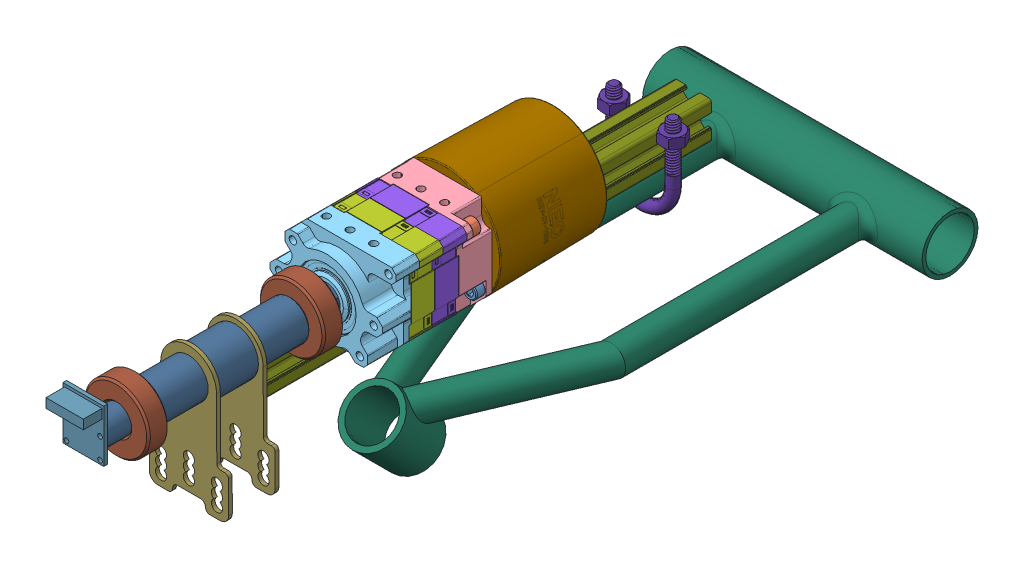
SolidWorks assembly SBW lower asm, configuration Default. Lengths in mm.
Overall size (161.8 159.3 415).
29 component instances, 20 part files, 63 mates.
Components (placement in the parent):
- MAXPlanetary 2-Stage-1: MAXPlanetary 2-Stage [Default] at origin size (89.61 89.51 122.08)
  - MAXPlanetary 2-Stage.STEP-1: MAXPlanetary 2-Stage.STEP [Default] at origin size (89.61 89.51 122.08)
    - REV-25-2109_2-Stage (No Shaft, For NEO).STEP-1: REV-25-2109_2-Stage (No Shaft, For NEO).STEP [Default] at origin size (65.15 54.03 73.34)
      - REV-25-2107_2-Stage.STEP-1: REV-25-2107_2-Stage.STEP [Default] at (0 0 6.35) x (-1 0 0) z (0 0 -1) size (65.15 54.03 73.34)
        - #10 Socket Head Cap Screws_0.500in Long.STEP-1: #10 Socket Head Cap Screws_0.500in Long.STEP [Default] at (21.1355 14.0872 12.7) x (0.923728 0.383049 0) z (0.383049 -0.923728 0) size (7.94 17.53 7.94)
        - #10 Socket Head Cap Screws_0.500in Long.STEP-2: #10 Socket Head Cap Screws_0.500in Long.STEP [Default] at (-21.1355 -14.0872 12.7) x (0.923728 0.383049 0) z (0.383049 -0.923728 0) size (7.94 17.53 7.94)
        - #10 Socket Head Cap Screws_1.500in Long.STEP-1: #10 Socket Head Cap Screws_1.500in Long.STEP [Default] at (-26.9919 21.4312 0) x (0.777574 0.628792 0) z (-0.628792 0.777574 0) size (7.94 42.93 7.94)
        - #10 Socket Head Cap Screws_1.500in Long.STEP-2: #10 Socket Head Cap Screws_1.500in Long.STEP [Default] at (26.9919 -21.4312 0) x (0.777574 0.628792 0) z (-0.628792 0.777574 0) size (7.94 42.93 7.94)
        - #10-32 Button Head Cap Screws_0.500in Long.STEP-1: #10-32 Button Head Cap Screws_0.500in Long.STEP [Default] at (0 0 -35.2425) x (0.655967 -0.754789 0) z (-0.754789 -0.655967 0) size (9.17 15.27 9.17)
      - REV-21-2106.STEP-1: REV-21-2106.STEP [Default] at origin size (61.91 50.8 19.05)
      - REV-21-2104.STEP-1: REV-21-2104.STEP [Default] at (0 0 44.45) x (0 0 1) z (-1 0 0) size (23.2 50.8 61.92)
      - REV-21-2108.STEP-1: REV-21-2108.STEP [Default] at (0 0 7.0985) x (-0.554615 -0.832107 0) z (0 0 -1) size (25.4 25.4 14.94)
    - REV-21-2101.STEP-1: REV-21-2101.STEP [Default] at (0 0 28.575) size (61.91 50.8 16.85)
    - REV-21-2102.STEP-1: REV-21-2102.STEP [Default] at (0 0 15.875) size (61.91 50.8 16.85)
    - REV-21-1650.STEP-1: REV-21-1650.STEP [Default] at (0 0 -9.525) x (0.554615 0.832107 0) z (0 0 1) size (64.41 64.76 93.26)
- shaft-1: shaft [Default] at (0 0 42.8625) x (0 0 1) z (-0.999764 0.021721 0) size (138 25 25)
- deep groove bearing 6202-1: deep groove bearing 6202 [默认] at (0 0 61.8625) size (35 35 11)
- shaft link-1: shaft link [默认] at (0 0 100.8625) x (0.999993 0.003842 0) z (0 0 1) size (42.5 73 2)
- shaft link-2: shaft link [默认] at (0 0 125.8625) x (0.999993 0.003842 0) z (0 0 1) size (42.5 73 2)
- AS5047P magnet-1: AS5047P magnet [Default] at (0 0 180.8625) x (1 0 0) z (0 1 0) size (6 2.5 6)
- deep groove bearing 6202-2: deep groove bearing 6202 [默认] at (0 0 155.8625) size (35 35 11)
- AS5047P-1: AS5047P [Default] at (0 6.4979 182.3625) size (22 28 12)
- lower AS5047P mount-1: lower AS5047P mount [Default] at (0 0 189.3625) x (0 0 -1) z (1 0 0) size (5 92.5 55) (hidden)
- BLDC mount 1-1: BLDC mount 1 [默认] at (0 0 53.975) size (60 95 5) (hidden)
- frame asm-1: frame asm [默认] at (0 -66.9754 29.3625) x (0 0 1) z (0 1 0) size (330 260 46.82)
  - sw frame-1: sw frame [默认] at (-220 0 -0.0001) x (-1 0 0) z (0 0 -1) size (260.61 150 46.82)
  - middle frame-1: middle frame [默认] at (65 -130 -10) x (1 0 0) z (0 1 0) size (30 30 260) (hidden)
- T-slot frame test-1: T-slot frame test [默认] at (-38 -48.9719 -180.6375) size (20 20 270)
- 3043T614_U-Bolt-1: 3043T614_U-Bolt [3043T614] at (-37.9982 -62.7708 -154.1666) size (44.58 51.3 11.11)
Mates (geometry in assembly coordinates):
- front: coincident aligned: plane of MAXPlanetary 2-Stage-1 through (0 0 0) normal (0 0 1)
- top: coincident aligned: plane of MAXPlanetary 2-Stage-1 through (0 0 0) normal (0 1 0)
- right: coincident aligned: plane of MAXPlanetary 2-Stage-1 through (0 0 0) normal (1 0 0)
- 重合2: coincident anti-aligned: plane of MAXPlanetary 2-Stage-1/MAXPlanetary 2-Stage.STEP-1/REV-25-2109_2-Stage (No Shaft, For NEO).STEP-1/REV-21-2104.STEP-1 through (0 0 42.8625) normal (0 0 1); plane of shaft-1 through (0 0 42.8625) normal (0 0 -1)
- 同心1: concentric anti-aligned: circle of MAXPlanetary 2-Stage-1/MAXPlanetary 2-Stage.STEP-1/REV-25-2109_2-Stage (No Shaft, For NEO).STEP-1/REV-21-2104.STEP-1; cylinder of shaft-1 through (0 0 72.8625) axis (0 0 -1) radius 7.5
- 平行1: parallel anti-aligned: plane of MAXPlanetary 2-Stage-1/MAXPlanetary 2-Stage.STEP-1/REV-25-2109_2-Stage (No Shaft, For NEO).STEP-1/REV-21-2104.STEP-1 through (0.1594 7.3379 42.8625) normal (0.481071 -0.876682 0); plane of shaft-1 through (0.1593 7.3306 57.8625) normal (-0.481071 0.876682 0)
- 同心2: concentric aligned: cylinder of shaft-1 through (0 0 72.8625) axis (0 0 -1) radius 7.5; cylinder of deep groove bearing 6202-1 through (0 0 72.8625) axis (0 0 -1) radius 7.5
- 重合3: coincident anti-aligned: plane of shaft-1 through (0 0 72.8625) normal (0 0 -1); plane of deep groove bearing 6202-1 through (0 0 72.8625) normal (0 0 1)
- 同心3: concentric aligned: cylinder of shaft-1 through (0 0 102.8625) axis (0 0 -1) radius 10.5; cylinder of shaft link-1 through (0 0 102.8625) axis (0 0 -1) radius 10.5
- 重合4: coincident anti-aligned: plane of shaft-1 through (0 0 102.8625) normal (0 0 -1); plane of shaft link-1 through (-11.0367 -55.5428 102.8625) normal (0 0 1)
- 同心4: concentric aligned: cylinder of shaft-1 through (0 0 155.8625) axis (0 0 -1) radius 10.5; cylinder of shaft link-2 through (0 0 127.8625) axis (0 0 -1) radius 10.5
- 重合5: coincident anti-aligned: plane of shaft-1 through (0 0 125.8625) normal (0 0 1); plane of shaft link-2 through (-11.0367 -55.5428 125.8625) normal (0 0 -1)
- 重合6: coincident aligned: plane of shaft link-1 through (-14.9999 -0.0576 102.8625) normal (-0.999993 -0.003842 0); plane of shaft link-2 through (-14.9999 -0.0576 127.8625) normal (-0.999993 -0.003842 0)
- 重合7: coincident anti-aligned: plane of shaft-1 through (0 0 178.3625) normal (0 0 1); plane of AS5047P magnet-1 through (0 0 178.3625) normal (0 0 -1)
- 同心5: concentric aligned: cylinder of shaft-1 through (0 0 178.3625) axis (0 0 1) radius 3.5; cylinder of AS5047P magnet-1 through (0 0 178.3625) axis (0 0 1) radius 3
- 同心6: concentric aligned: cylinder of shaft-1 through (0 0 180.8625) axis (0 0 -1) radius 7.5; cylinder of deep groove bearing 6202-2 through (0 0 166.8625) axis (0 0 -1) radius 7.5
- 重合8: coincident anti-aligned: plane of shaft-1 through (0 0 155.8625) normal (0 0 1); plane of deep groove bearing 6202-2 through (0 0 155.8625) normal (0 0 -1)
- 距离1: distance = 1.5 mm anti-aligned: plane of AS5047P-1 through (0 6.4979 182.3625) normal (0 0 -1); plane of AS5047P magnet-1 through (0 0 180.8625) normal (0 0 1)
- 同心7: concentric: cylinder of AS5047P magnet-1 through (0 0 178.3625) axis (0 0 1) radius 3; point of AS5047P-1
- 平行4: parallel aligned: plane of MAXPlanetary 2-Stage-1/MAXPlanetary 2-Stage.STEP-1/REV-25-2109_2-Stage (No Shaft, For NEO).STEP-1/REV-21-2104.STEP-1 through (-30.1625 0 23.2597) normal (-1 0 0); plane of AS5047P-1 through (-11 20.4979 184.3625) normal (-1 0 0)
- 重合15: coincident anti-aligned: plane of AS5047P-1 through (0 6.4979 184.3625) normal (0 0 1); plane of lower AS5047P mount-1 through (0 0 184.3625) normal (0 0 -1)
- 同心8: concentric aligned: cylinder of AS5047P-1 through (-9 5.5 184.3625) axis (0 0 -1) radius 1.3; cylinder of lower AS5047P mount-1 through (-9 5.5 189.3625) axis (0 0 -1) radius 1.4
- 同心9: concentric aligned: cylinder of AS5047P-1 through (9 -5.5 184.3625) axis (0 0 -1) radius 1.3; cylinder of lower AS5047P mount-1 through (9 -5.5 189.3625) axis (0 0 -1) radius 1.4
- 同心10: concentric aligned: cylinder of shaft-1 through (0 0 72.8625) axis (0 0 -1) radius 7.5; cylinder of BLDC mount 1-1 through (0 0 58.975) axis (0 0 -1) radius 12.5
- 同心11: concentric anti-aligned: cylinder of MAXPlanetary 2-Stage-1/MAXPlanetary 2-Stage.STEP-1/REV-25-2109_2-Stage (No Shaft, For NEO).STEP-1/REV-21-2104.STEP-1 through (-17.9605 17.9605 53.975) axis (0 0 1) radius 2.0193; cylinder of BLDC mount 1-1 through (-17.96 17.96 58.975) axis (0 0 -1) radius 2
- 重合16: coincident anti-aligned: plane of MAXPlanetary 2-Stage-1/MAXPlanetary 2-Stage.STEP-1/REV-25-2109_2-Stage (No Shaft, For NEO).STEP-1/REV-21-2104.STEP-1 through (0 0 53.975) normal (0 0 1); plane of BLDC mount 1-1 through (0 0 53.975) normal (0 0 -1)
- 距离2: distance = 130 mm: plane of assembly through (0 0 0) normal (1 0 0); plane of assembly; plane of middle frame-1 through (130 -110.5456 57.9191) normal (1 0 0)
- 距离8: distance = 55 mm aligned: plane of sw frame-1 through (-75 -118.6918 -247.8837) normal (-1 0 0); plane of middle frame-1 through (-130 -110.5456 57.9191) normal (-1 0 0)
- 重合18: coincident anti-aligned: plane of sw frame-2 through (0 -92 -125.6375) normal (-1 0 0)
- 同心12: concentric anti-aligned: cylinder of sw frame-2 through (0 -107 94.3625) axis (0 1 0) radius 13
- 重合21: coincident: plane of sw frame-2 through (0 -77 94.3625) normal (0 1 0)
- 重合22: coincident aligned: plane of frame asm-1 through (0 -66.9754 29.3625) normal (1 0 0)
- 平行7: parallel aligned: plane of frame asm-1 through (0 -66.9754 29.3625) normal (0 0 1)
- 距离9: distance = 11.5 mm: plane of assembly; plane of frame asm-1; plane of shaft link-1 through (-11.0367 -55.5428 102.8625) normal (0 0 1)
- 相切1: tangent anti-aligned: cylinder of frame asm-1/sw frame-1 through (-38 -66.9754 -60.6375) axis (0 0 -1) radius 8; plane of 8875T911_Mount Plate for 1 4 -20 Thread Size-1 through (-58.6375 -58.9742 -180.6375) normal (0 -1 0)
- 平行8: parallel aligned: plane of 8875T911_Mount Plate for 1 4 -20 Thread Size-1 through (-58.6375 -56.5929 -180.6375) normal (0 1 0)
- 平行9: parallel anti-aligned: plane of 8875T911_Mount Plate for 1 4 -20 Thread Size-1 through (-17.3625 -56.5929 -180.6375) normal (0 0 -1)
- 同心14: concentric anti-aligned: cylinder of 8875T911_Mount Plate for 1 4 -20 Thread Size-1 through (-50.7 -56.5929 -171.1125) axis (0 -1 0) radius 3.175; cylinder of 8875T911_Mount Plate for 1 4 -20 Thread Size-2 through (-50.7 -36.5884 -171.1125) axis (0 1 0) radius 3.175
- 同心15: concentric anti-aligned: cylinder of 8875T911_Mount Plate for 1 4 -20 Thread Size-1 through (-25.3 -56.5929 -171.1125) axis (0 -1 0) radius 3.175; cylinder of 8875T911_Mount Plate for 1 4 -20 Thread Size-2 through (-25.3 -36.5884 -171.1125) axis (0 1 0) radius 3.175
- 重合25: coincident anti-aligned: plane of T-slot frame test-1 through (-38 -58.9742 89.3625) normal (0 -1 0); plane of 8875T911_Mount Plate for 1 4 -20 Thread Size-1 through (-58.6375 -56.5929 -180.6375) normal (0 1 0)
- 平行10: parallel aligned: cylinder of frame asm-1/sw frame-1 through (-38 -66.9754 -60.6375) axis (0 0 -1) radius 6; cylinder of T-slot frame test-1 through (-38 -48.9719 89.3625) axis (0 0 -1) radius 2.5
- 重合26: coincident anti-aligned: plane of T-slot frame test-1 through (-38 -38.9697 89.3625) normal (0 1 0); plane of 8875T911_Mount Plate for 1 4 -20 Thread Size-2 through (-17.3625 -36.5884 -180.6375) normal (0 -1 0)
- 距离11: distance = 10 mm anti-aligned: plane of T-slot frame test-1 through (-38 -48.9719 -180.6375) normal (0 0 -1); cylinder of frame asm-1/sw frame-1 through (75 -66.9754 -205.6375) axis (-1 0 0) radius 15
- 重合27: coincident aligned: plane of T-slot frame test-1 through (-38 -48.9719 -180.6375) normal (0 0 -1); plane of 8875T911_Mount Plate for 1 4 -20 Thread Size-2 through (-58.6375 -36.5884 -180.6375) normal (0 0 -1)
- 距离12: distance = 0 mm: plane of 8875T911_Mount Plate for 1 4 -20 Thread Size-2 through (-38 -34.2072 -171.1125) normal (-1 0 0); cylinder of T-slot frame test-1 through (-38 -48.9719 89.3625) axis (0 0 -1) radius 2.5
- 距离13: distance = 0 mm: plane of T-slot frame test-1 through (-38 -48.9719 -180.6375) normal (1 0 0); cylinder of frame asm-1/sw frame-1 through (-38 -66.9754 -60.6375) axis (0 0 -1) radius 8
- 重合28: coincident aligned: plane of 8875T911_Mount Plate for 1 4 -20 Thread Size-1 through (-58.6375 -56.5929 -161.5875) normal (-1 0 0); plane of 8875T911_Mount Plate for 1 4 -20 Thread Size-3 through (-58.6375 -58.9742 -79.6875) normal (-1 0 0)
- 重合29: coincident aligned: plane of 8875T911_Mount Plate for 1 4 -20 Thread Size-1 through (-58.6375 -56.5929 -180.6375) normal (0 1 0); plane of 8875T911_Mount Plate for 1 4 -20 Thread Size-3 through (-58.6375 -56.5929 -60.6375) normal (0 1 0)
- 重合30: coincident anti-aligned: circle of frame asm-1/sw frame-1; plane of 8875T911_Mount Plate for 1 4 -20 Thread Size-3 through (-17.3625 -58.9742 -60.6375) normal (0 0 1)
- 重合31: coincident aligned: plane of 8875T911_Mount Plate for 1 4 -20 Thread Size-2 through (-17.3625 -34.2072 -180.6375) normal (0 1 0); plane of 8875T911_Mount Plate for 1 4 -20 Thread Size-4 through (-17.3625 -34.2072 -79.6875) normal (0 1 0)
- 重合32: coincident aligned: plane of 8875T911_Mount Plate for 1 4 -20 Thread Size-3 through (-58.6375 -58.9742 -79.6875) normal (-1 0 0); plane of 8875T911_Mount Plate for 1 4 -20 Thread Size-4 through (-58.6375 -36.5884 -60.6375) normal (-1 0 0)
- 重合33: coincident aligned: plane of 8875T911_Mount Plate for 1 4 -20 Thread Size-3 through (-17.3625 -58.9742 -79.6875) normal (0 0 -1); plane of 8875T911_Mount Plate for 1 4 -20 Thread Size-4 through (-58.6375 -36.5884 -79.6875) normal (0 0 -1)
- 相切2: tangent aligned: cylinder of frame asm-1/sw frame-1 through (-38 -66.9754 -60.6375) axis (0 0 -1) radius 8; plane of 8875T914_Mount Plate for 3 8 -16 Thread Size-1 through (-9.425 -58.9742 -180.6375) normal (0 1 0)
- 重合34: coincident aligned: plane of T-slot frame test-1 through (-38 -48.9719 -180.6375) normal (0 0 -1); plane of 8875T914_Mount Plate for 3 8 -16 Thread Size-1 through (-66.575 -62.1492 -180.6375) normal (0 0 -1)
- 距离14: distance = 0 mm: plane of 8875T914_Mount Plate for 3 8 -16 Thread Size-1 through (-38 -58.9742 -167.9375) normal (-1 0 0); cylinder of frame asm-1/sw frame-1 through (-38 -66.9754 -60.6375) axis (0 0 -1) radius 8
- 平行11: parallel aligned: plane of 8875T914_Mount Plate for 3 8 -16 Thread Size-1 through (-9.425 -58.9742 -180.6375) normal (0 1 0)
- 重合36: coincident anti-aligned: plane of T-slot frame test-1 through (-38 -58.9742 89.3625) normal (0 -1 0); plane of 8875T914_Mount Plate for 3 8 -16 Thread Size-1 through (-9.425 -58.9742 -180.6375) normal (0 1 0)
- 同心16: concentric aligned: cylinder of 8875T914_Mount Plate for 3 8 -16 Thread Size-1 through (-20.5375 -62.1492 -167.9375) axis (0 1 0) radius 4.7625; cylinder of U-shape bolt-1 through (-20.5375 -70.2447 -167.9375) axis (0 1 0) radius 4.7625
- 同心17: concentric aligned: cylinder of 8875T914_Mount Plate for 3 8 -16 Thread Size-1 through (-55.4625 -62.1492 -167.9375) axis (0 1 0) radius 4.7625; cylinder of U-shape bolt-1 through (-55.4625 -57.5447 -167.9375) axis (0 1 0) radius 4.7625
- 重合37: coincident anti-aligned: plane of T-slot frame test-1 through (-38 -38.9697 89.3625) normal (0 1 0); plane of 8875T914_Mount Plate for 3 8 -16 Thread Size-2 through (-66.575 -38.9697 -180.6375) normal (0 -1 0)
- 重合38: coincident aligned: plane of 8875T914_Mount Plate for 3 8 -16 Thread Size-1 through (-66.575 -62.1492 -180.6375) normal (0 0 -1); plane of 8875T914_Mount Plate for 3 8 -16 Thread Size-2 through (-9.425 -35.7947 -180.6375) normal (0 0 -1)
- 重合39: coincident aligned: plane of 8875T914_Mount Plate for 3 8 -16 Thread Size-1 through (-66.575 -62.1492 -155.2375) normal (-1 0 0); plane of 8875T914_Mount Plate for 3 8 -16 Thread Size-2 through (-66.575 -35.7947 -155.2375) normal (-1 0 0)
- 距离15: distance = 10 mm aligned: plane of U-shape bolt-1 through (-20.5375 -25.7947 -167.9375) normal (0 1 0); plane of 8875T914_Mount Plate for 3 8 -16 Thread Size-2 through (-66.575 -35.7947 -180.6375) normal (0 1 0)
